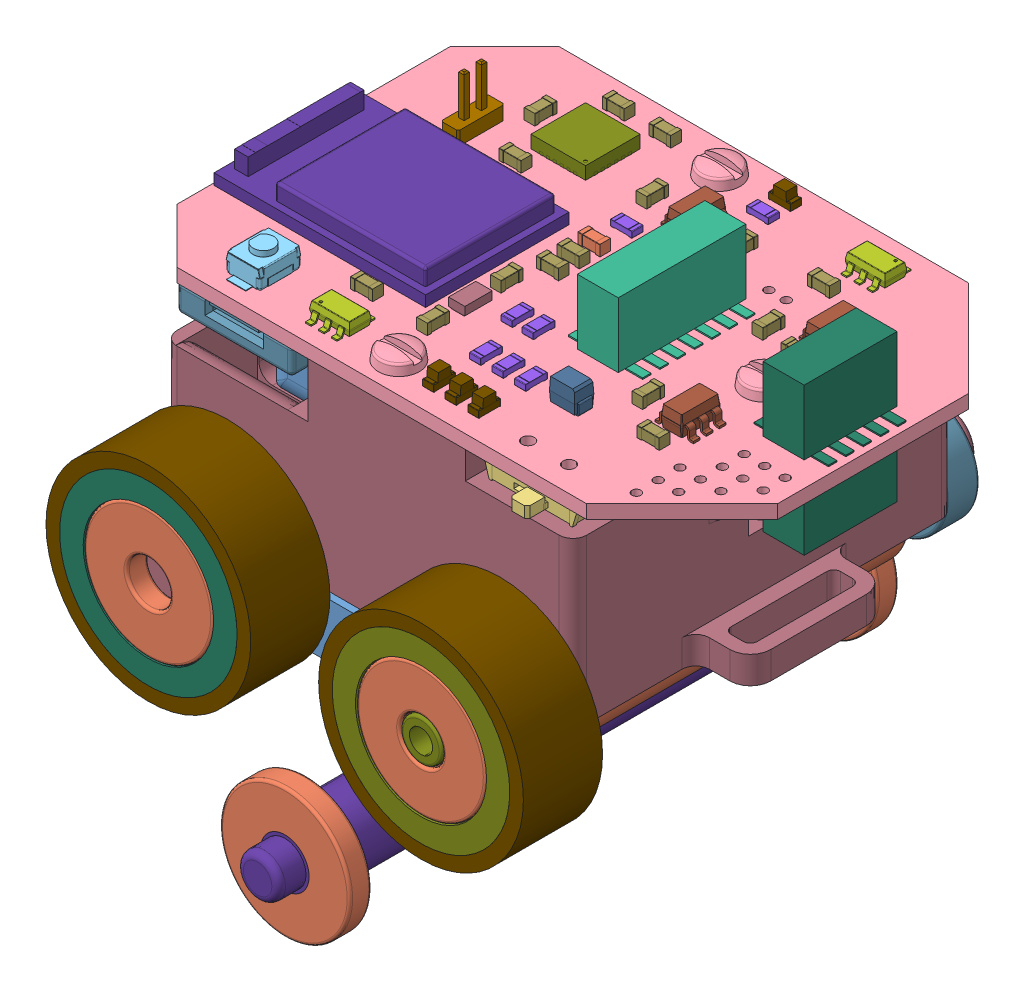
SolidWorks assembly AstroAnt_small_magnet, configuration Default. Lengths in mm.
Overall size (41 37.39 42.61).
158 component instances, 38 part files, 36 mates.
Components (placement in the parent):
- LiPo_360mAh-1: LiPo_360mAh [Default] at (6.8166 4.9998 44.2756) size (25 7 18)
- PA2-50-1: PA2-50 [Default] at (8.0673 -18.301 41.8029) x (0 0 1) z (0.952879 0.303349 0) size (29.1 8 8)
- PA2-50-2: PA2-50 [Default] at (-4.1563 19.5334 49.6029) x (0 0 -1) z (0.755989 -0.654584 0) size (29.1 8 8)
- 92120A150_Brass Heat-Set Inserts for Plastic-1: 92120A150_Brass Heat-Set Inserts for Plastic [92120A150] at (19.9543 12.4998 45.7029) size (2.56 3.33 2.56)
- 92120A150_Brass Heat-Set Inserts for Plastic-2: 92120A150_Brass Heat-Set Inserts for Plastic [92120A150] at (4.9543 12.4998 33.9529) size (2.56 3.33 2.56)
- 92120A150_Brass Heat-Set Inserts for Plastic-3: 92120A150_Brass Heat-Set Inserts for Plastic [92120A150] at (4.9543 12.4998 57.4529) size (2.56 3.33 2.56)
- 91460A005_METRIC CHEESE HEAD SLOTTED MACHINE SCREW-8: 91460A005_METRIC CHEESE HEAD SLOTTED MACHINE SCREW [91460A005] at (4.9543 14.9998 57.4529) x (1 0 0) z (0 1 0) size (3 3 7.1)
- 91460A005_METRIC CHEESE HEAD SLOTTED MACHINE SCREW-9: 91460A005_METRIC CHEESE HEAD SLOTTED MACHINE SCREW [91460A005] at (4.9543 14.9998 33.9529) x (1 0 0) z (0 1 0) size (3 3 7.1)
- 91460A005_METRIC CHEESE HEAD SLOTTED MACHINE SCREW-10: 91460A005_METRIC CHEESE HEAD SLOTTED MACHINE SCREW [91460A005] at (19.9543 14.9998 45.7029) x (1 0 0) z (0 1 0) size (3 3 7.1)
- 92120A150_Brass Heat-Set Inserts for Plastic-4: 92120A150_Brass Heat-Set Inserts for Plastic [92120A150] at (4.9543 1.4998 57.4529) x (-0.616962 0 -0.786993) z (0.786993 0 -0.616962) size (2.56 3.33 2.56)
- 92120A150_Brass Heat-Set Inserts for Plastic-5: 92120A150_Brass Heat-Set Inserts for Plastic [92120A150] at (4.9543 1.4998 33.9529) x (-0.616962 0 -0.786993) z (0.786993 0 -0.616962) size (2.56 3.33 2.56)
- 91460A005_METRIC CHEESE HEAD SLOTTED MACHINE SCREW-14: 91460A005_METRIC CHEESE HEAD SLOTTED MACHINE SCREW [91460A005] at (4.9543 -2.5002 57.4529) x (0.663599 0 0.748089) z (0 -1 0) size (3 3 7.1)
- 91460A005_METRIC CHEESE HEAD SLOTTED MACHINE SCREW-15: 91460A005_METRIC CHEESE HEAD SLOTTED MACHINE SCREW [91460A005] at (4.9543 -2.5002 33.9529) x (0.663599 0 0.748089) z (0 -1 0) size (3 3 7.1)
- mainboard_v1.step-1: mainboard_v1.step [Default] at (-103.0457 13.9998 235.7029) x (0 0 -1) z (0 1 0) size (29.41 41 10.8)
  - B3U-1000P.step-1: B3U-1000P.step [Default] at (178.95 -97.38 1.05) x (1 0 0) z (0 -1 0) size (4 1.75 2.5)
    - COMPOUND.step-1: COMPOUND.step [Default] at origin size (4 1.75 2.5)
  - 20021321-00014C1LF.step-1: 20021321-00014C1LF.step [Default] at (190 -115.5 1.05) size (9.35 5.45 4.85)
    - COMPOUND-0.step-1: COMPOUND-0.step [Default] at origin size (9.35 5.45 4.85)
  - MP6513GJ-Z.step-1: MP6513GJ-Z.step [Default] at (201.21 -120 1.05) x (-1 0 0) z (0 0 1) size (2.8 2.9 1)
    - COMPOUND-1.step-1: COMPOUND-1.step [Default] at origin size (2.8 2.9 1)
  - MP6513GJ-Z.step-2: MP6513GJ-Z.step [Default] at (178.51 -103.46 1.05) size (2.8 2.9 1)
    - COMPOUND-1.step-1: COMPOUND-1.step [Default] at origin size (2.8 2.9 1)
  - R_0603_1608Metric.step-1: R_0603_1608Metric.step [Default] at (195.55 -104.38 -0.05) x (1 0 0) z (0 0 -1) size (1.6 0.8 0.45)
    - SOLID.step-1: SOLID.step [Default] at origin size (1.6 0.8 0.45)
  - R_0603_1608Metric.step-2: R_0603_1608Metric.step [Default] at (192.6 -99.86 -0.05) x (0 1 0) z (0 0 -1) size (1.6 0.8 0.45)
    - SOLID.step-1: SOLID.step [Default] at origin size (1.6 0.8 0.45)
  - PinHeader_2x01_P1.27mm_Vertical.step-1: PinHeader_2x01_P1.27mm_Vertical.step [Default] at (194.96 -96.07 1.05) size (3.4 1.27 6.3)
    - SOLID-2.step-1: SOLID-2.step [Default] at origin size (3.4 1.27 6.3)
  - TAJP106K010RNJ.step-1: TAJP106K010RNJ.step [Default] at (196.22 -98.14 -0.05) x (-1 0 0) z (0 0 -1) size (2.05 1.4 1.7)
    - COMPOUND-3.step-1: COMPOUND-3.step [Default] at origin size (2.05 1.4 1.7)
  - TAJP106K010RNJ.step-2: TAJP106K010RNJ.step [Default] at (181.68 -117.23 1.05) x (0 1 0) z (0 0 1) size (2.05 1.4 1.7)
    - COMPOUND-3.step-1: COMPOUND-3.step [Default] at origin size (2.05 1.4 1.7)
  - SOT-23-5.step-1: SOT-23-5.step [Default] at (195.38 -122.78 1.05) x (0 1 0) z (0 0 1) size (2.8 2.9 1.55)
    - SOLID-4.step-1: SOLID-4.step [Default] at origin size (2.8 2.9 1.55)
  - C_0603_1608Metric.step-1: C_0603_1608Metric.step [Default] at (192.91 -122.55 1.05) x (0 -1 0) z (0 0 1) size (1.6 0.8 0.8)
    - SOLID-5.step-1: SOLID-5.step [Default] at origin size (1.6 0.8 0.8)
  - C_0603_1608Metric.step-2: C_0603_1608Metric.step [Default] at (193.57 -119.76 1.05) size (1.6 0.8 0.8)
    - SOLID-5.step-1: SOLID-5.step [Default] at origin size (1.6 0.8 0.8)
  - ECS-.327-12.5-12-TR.step-1: ECS-.327-12.5-12-TR.step [Default] at (184.31 -107.18 1.05) size (2 1.2 0.7)
    - COMPOUND-6.step-1: COMPOUND-6.step [Default] at origin size (2 1.2 0.7)
  - C_0603_1608Metric.step-3: C_0603_1608Metric.step [Default] at (197.67 -113.69 1.05) size (1.6 0.8 0.8)
    - SOLID-5.step-1: SOLID-5.step [Default] at origin size (1.6 0.8 0.8)
  - C_0603_1608Metric.step-4: C_0603_1608Metric.step [Default] at (197.64 -107.18 1.05) size (1.6 0.8 0.8)
    - SOLID-5.step-1: SOLID-5.step [Default] at origin size (1.6 0.8 0.8)
  - C_0603_1608Metric.step-5: C_0603_1608Metric.step [Default] at (190.96 -108.09 1.05) x (0 1 0) z (0 0 1) size (1.6 0.8 0.8)
    - SOLID-5.step-1: SOLID-5.step [Default] at origin size (1.6 0.8 0.8)
  - 1734592-6.step-1: 1734592-6.step [Default] at (203.79 -118 -1.05) x (0 -1 0) z (1 0 0) size (8.43 2.05 5.11)
    - SOLID-7.step-1: SOLID-7.step [Default] at origin size (8.43 2.05 5.11)
  - 1734592-6.step-2: 1734592-6.step [Default] at (176.19 -98 -1.05) x (0 1 0) z (-1 0 0) size (8.43 2.05 5.11)
    - SOLID-7.step-1: SOLID-7.step [Default] at origin size (8.43 2.05 5.11)
  - 20021321-00010C4LF.step-1: 20021321-00010C4LF.step [Default] at (190 -127.85 -0.05) x (1 0 0) z (0 0 -1) size (6.81 5.45 4.85)
    - COMPOUND-8.step-1: COMPOUND-8.step [Default] at origin size (6.81 5.45 4.85)
  - 20021321-00010C4LF.step-2: 20021321-00010C4LF.step [Default] at (190 -127.85 1.05) size (6.81 5.45 4.85)
    - COMPOUND-8.step-1: COMPOUND-8.step [Default] at origin size (6.81 5.45 4.85)
  - C_0603_1608Metric.step-6: C_0603_1608Metric.step [Default] at (181.31 -102.6 1.05) x (0 -1 0) z (0 0 1) size (1.6 0.8 0.8)
    - SOLID-5.step-1: SOLID-5.step [Default] at origin size (1.6 0.8 0.8)
  - C_0603_1608Metric.step-7: C_0603_1608Metric.step [Default] at (198.25 -119.14 1.05) x (0 -1 0) z (0 0 1) size (1.6 0.8 0.8)
    - SOLID-5.step-1: SOLID-5.step [Default] at origin size (1.6 0.8 0.8)
  - MPU6050.step-1: MPU6050.step [Default] at (198.43 -101.5 1.05) x (0 1 0) z (1 0 0) size (4 0.95 4)
    - COMPOUND-9.step-1: COMPOUND-9.step [Default] at origin size (4 0.95 4)
  - C_0603_1608Metric.step-8: C_0603_1608Metric.step [Default] at (194.9 -99.89 1.05) x (0 -1 0) z (0 0 1) size (1.6 0.8 0.8)
    - SOLID-5.step-1: SOLID-5.step [Default] at origin size (1.6 0.8 0.8)
  - C_0603_1608Metric.step-9: C_0603_1608Metric.step [Default] at (201.98 -100.38 1.05) x (0 -1 0) z (0 0 1) size (1.6 0.8 0.8)
    - SOLID-5.step-1: SOLID-5.step [Default] at origin size (1.6 0.8 0.8)
  - C_0603_1608Metric.step-10: C_0603_1608Metric.step [Default] at (201.98 -103.78 1.05) x (0 1 0) z (0 0 1) size (1.6 0.8 0.8)
    - SOLID-5.step-1: SOLID-5.step [Default] at origin size (1.6 0.8 0.8)
  - C_0603_1608Metric.step-11: C_0603_1608Metric.step [Default] at (198.81 -97.82 1.05) size (1.6 0.8 0.8)
    - SOLID-5.step-1: SOLID-5.step [Default] at origin size (1.6 0.8 0.8)
  - SOT-23-5.step-2: SOT-23-5.step [Default] at (184.86 -122.77 1.05) x (0 1 0) z (0 0 1) size (2.8 2.9 1.55)
    - SOLID-4.step-1: SOLID-4.step [Default] at origin size (2.8 2.9 1.55)
  - SOT-23-5.step-3: SOT-23-5.step [Default] at (197.58 -110.46 1.05) x (0 1 0) z (0 0 1) size (2.8 2.9 1.55)
    - SOLID-4.step-1: SOLID-4.step [Default] at origin size (2.8 2.9 1.55)
  - MDBT50Q-1MV2.step-1: MDBT50Q-1MV2.step [Default] at (187.3136 -98.605 1.0754) x (-1 0 0) z (0 1 0) size (10.5 2.06 15.5)
    - SOLID-10.step-1: SOLID-10.step [Default] at origin size (10.5 2.06 15.5)
  - C_0603_1608Metric.step-12: C_0603_1608Metric.step [Default] at (189.44 -108.09 1.05) x (0 1 0) z (0 0 1) size (1.6 0.8 0.8)
    - SOLID-5.step-1: SOLID-5.step [Default] at origin size (1.6 0.8 0.8)
  - C_0603_1608Metric.step-13: C_0603_1608Metric.step [Default] at (181.57 -107.18 1.05) x (-1 0 0) z (0 0 1) size (1.6 0.8 0.8)
    - SOLID-5.step-1: SOLID-5.step [Default] at origin size (1.6 0.8 0.8)
  - C_0603_1608Metric.step-14: C_0603_1608Metric.step [Default] at (186.97 -107.18 1.05) size (1.6 0.8 0.8)
    - SOLID-5.step-1: SOLID-5.step [Default] at origin size (1.6 0.8 0.8)
  - C_0603_1608Metric.step-15: C_0603_1608Metric.step [Default] at (184.77 -119.75 1.05) x (-1 0 0) z (0 0 1) size (1.6 0.8 0.8)
    - SOLID-5.step-1: SOLID-5.step [Default] at origin size (1.6 0.8 0.8)
  - C_0603_1608Metric.step-16: C_0603_1608Metric.step [Default] at (182.37 -122.54 1.05) x (0 -1 0) z (0 0 1) size (1.6 0.8 0.8)
    - SOLID-5.step-1: SOLID-5.step [Default] at origin size (1.6 0.8 0.8)
  - LED_0603_1608Metric.step-1: LED_0603_1608Metric.step [Default] at (178.19 -111.01 1.05) size (1.6 0.8 1.1)
    - SOLID-11.step-1: SOLID-11.step [Default] at origin size (1.6 0.8 1.1)
  - LED_0603_1608Metric.step-2: LED_0603_1608Metric.step [Default] at (178.19 -112.66 1.05) size (1.6 0.8 1.1)
    - SOLID-11.step-1: SOLID-11.step [Default] at origin size (1.6 0.8 1.1)
  - LED_0603_1608Metric.step-3: LED_0603_1608Metric.step [Default] at (178.19 -114.31 1.05) size (1.6 0.8 1.1)
    - SOLID-11.step-1: SOLID-11.step [Default] at origin size (1.6 0.8 1.1)
  - LED_0603_1608Metric.step-4: LED_0603_1608Metric.step [Default] at (202.34 -112.21 1.05) x (0 1 0) z (0 0 1) size (1.6 0.8 1.1)
    - SOLID-11.step-1: SOLID-11.step [Default] at origin size (1.6 0.8 1.1)
  - 473460001.step-1: 473460001.step [Default] at (201.68 -99.72 -1.25) x (0 -1 0) z (1 0 0) size (7.98 2.94 5.43)
    - COMPOUND-12.step-1: COMPOUND-12.step [Default] at origin size (7.98 2.94 5.43)
  - L_0603_1608Metric.step-1: L_0603_1608Metric.step [Default] at (192.48 -108.09 1.05) x (0 1 0) z (0 0 1) size (1.6 0.8 0.8)
    - SOLID-13.step-1: SOLID-13.step [Default] at origin size (1.6 0.8 0.8)
  - R_0603_1608Metric.step-3: R_0603_1608Metric.step [Default] at (185.18 -111.31 1.05) x (-1 0 0) z (0 0 1) size (1.6 0.8 0.45)
    - SOLID.step-1: SOLID.step [Default] at origin size (1.6 0.8 0.45)
  - R_0603_1608Metric.step-4: R_0603_1608Metric.step [Default] at (185.18 -109.77 1.05) size (1.6 0.8 0.45)
    - SOLID.step-1: SOLID.step [Default] at origin size (1.6 0.8 0.45)
  - R_0603_1608Metric.step-5: R_0603_1608Metric.step [Default] at (181.62 -111.01 1.05) size (1.6 0.8 0.45)
    - SOLID.step-1: SOLID.step [Default] at origin size (1.6 0.8 0.45)
  - R_0603_1608Metric.step-6: R_0603_1608Metric.step [Default] at (181.62 -112.66 1.05) size (1.6 0.8 0.45)
    - SOLID.step-1: SOLID.step [Default] at origin size (1.6 0.8 0.45)
  - R_0603_1608Metric.step-7: R_0603_1608Metric.step [Default] at (181.62 -114.31 1.05) x (-1 0 0) z (0 0 1) size (1.6 0.8 0.45)
    - SOLID.step-1: SOLID.step [Default] at origin size (1.6 0.8 0.45)
  - R_0603_1608Metric.step-8: R_0603_1608Metric.step [Default] at (194.84 -108.1 1.05) x (0 1 0) z (0 0 1) size (1.6 0.8 0.45)
    - SOLID.step-1: SOLID.step [Default] at origin size (1.6 0.8 0.45)
  - R_0603_1608Metric.step-9: R_0603_1608Metric.step [Default] at (200.69 -112.2325 1.05) x (0 1 0) z (0 0 1) size (1.6 0.8 0.45)
    - SOLID.step-1: SOLID.step [Default] at origin size (1.6 0.8 0.45)
  - R_0603_1608Metric.step-10: R_0603_1608Metric.step [Default] at (196.22 -101.51 -0.05) x (-1 0 0) z (0 0 -1) size (1.6 0.8 0.45)
    - SOLID.step-1: SOLID.step [Default] at origin size (1.6 0.8 0.45)
  - R_0603_1608Metric.step-11: R_0603_1608Metric.step [Default] at (196.22 -99.9725 -0.05) x (-1 0 0) z (0 0 -1) size (1.6 0.8 0.45)
    - SOLID.step-1: SOLID.step [Default] at origin size (1.6 0.8 0.45)
  - SW_SPDT_PCM12.step-1: SW_SPDT_PCM12.step [Default] at (178.18 -119.37 -0.05) x (0 1 0) z (0 0 -1) size (7.7 5 2)
    - SOLID-14.step-1: SOLID-14.step [Default] at origin size (7.7 5 2)
  - COMPOUND-15.step-1: COMPOUND-15.step [Default] at origin size (28 41 1)
- 91613A020_METRIC CHEESE HEAD SLOTTED MACHINE SCREW-1: 91613A020_METRIC CHEESE HEAD SLOTTED MACHINE SCREW [91613A020] at (1.2533 -0.5002 54.4029) x (1 0 0) z (0 1 0) size (3 3 5.08)
- 91613A020_METRIC CHEESE HEAD SLOTTED MACHINE SCREW-2: 91613A020_METRIC CHEESE HEAD SLOTTED MACHINE SCREW [91613A020] at (8.6533 -0.5002 54.4029) x (1 0 0) z (0 1 0) size (3 3 5.08)
- 91613A020_METRIC CHEESE HEAD SLOTTED MACHINE SCREW-3: 91613A020_METRIC CHEESE HEAD SLOTTED MACHINE SCREW [91613A020] at (1.2533 -0.5002 37.0029) x (1 0 0) z (0 1 0) size (3 3 5.08)
- IR_TEMP_V2.step-3: IR_TEMP_V2.step [Default] at (118.9553 -0.5002 109.7029) x (-1 0 0) z (0 1 0) size (10 20 4.8)
  - Board_Geoms_380f.step-1: Board_Geoms_380f.step [Default] at origin size (10 20 1.11)
    - Pcb_380f.step-1: Pcb_380f.step [Default] at origin size (10 20 1)
    - topTracks_380f.step-1: topTracks_380f.step [Default] at (0 0 0.01) size (9.62 17.53 0.05)
    - botTracks_380f.step-1: botTracks_380f.step [Default] at (0 0 -1.01) size (9.25 16.88 0.05)
  - Step_Models_380f.step-1: Step_Models_380f.step [Default] at origin size (9.46 10.17 4.8)
    - Top_380f.step-1: Top_380f.step [Default] at origin size (9.46 10.17 1.2)
      - IC1_PW14_613E6C6D.step-1: IC1_PW14_613E6C6D.step [Default] at (113.99 -59.48 0) x (-1 0 0) z (0 1 0) size (6.4 1.2 5)
      - C1_C_0402_1005Metric_613EDDF6.step-1: C1_C_0402_1005Metric_613EDDF6.step [Default] at (110.5 -64.26 0) x (-1 0 0) z (0 0 1) size (1 0.5 0.5)
      - C1_C_0402_1005Metric_613EDDF6.step-2: C1_C_0402_1005Metric_613EDDF6.step [Default] at (109.52 -61.07 0) x (0 -1 0) z (0 0 1) size (1 0.5 0.5)
      - C1_C_0402_1005Metric_613EDDF6.step-3: C1_C_0402_1005Metric_613EDDF6.step [Default] at (118.48 -60.86 0) x (0 -1 0) z (0 0 1) size (1 0.5 0.5)
      - C1_C_0402_1005Metric_613EDDF6.step-4: C1_C_0402_1005Metric_613EDDF6.step [Default] at (118.48 -58.59 0) x (0 -1 0) z (0 0 1) size (1 0.5 0.5)
      - C1_C_0402_1005Metric_613EDDF6.step-5: C1_C_0402_1005Metric_613EDDF6.step [Default] at (113.32 -66.9 0) size (1 0.5 0.5)
      - R1_R_0402_1005Metric_613EDE7A.step-1: R1_R_0402_1005Metric_613EDE7A.step [Default] at (110.98 -63.1 0) size (1 0.5 0.35)
      - R1_R_0402_1005Metric_613EDE7A.step-2: R1_R_0402_1005Metric_613EDE7A.step [Default] at (111.68 -66.3 0) x (0 1 0) z (0 0 1) size (1 0.5 0.35)
    - Bot_380f.step-1: Bot_380f.step [Default] at origin size (6.35 7.64 4.6)
      - U1_ZTP-135SR_613E6CD4.step-1: U1_ZTP-135SR_613E6CD4.step [Default] at (114 -64 -1) x (-1 0 0) z (0 -1 0) size (6.35 4.6 5.4)
      - C1_C_0402_1005Metric_613EDDF6.step-1: C1_C_0402_1005Metric_613EDDF6.step [Default] at (115.07 -59.56 -1) x (0 -1 0) z (0 0 -1) size (1 0.5 0.5)
      - R1_R_0402_1005Metric_613EDE7A.step-1: R1_R_0402_1005Metric_613EDE7A.step [Default] at (113.64 -59.58 -1) x (0 -1 0) z (0 0 -1) size (1 0.5 0.35)
- Body_simple-1: Body_simple [Default] at (4.8007 -0.0002 38.7677) size (34 16 37)
- ball_bearing_5x11x4mm-1: ball_bearing_5x11x4mm [Default] at (-45.4624 -2.1758 28.9029) x (0.999925 -0.012245 0) z (0 0 1) size (8 8 2.5)
- wheel_holder_non_motor-1: wheel_holder_non_motor [Default] at (-70.2522 1.7638 25.6029) size (13 13 5.8) (hidden)
- wheel_holder_non_motor-2: wheel_holder_non_motor [Default] at (-19.1131 -84.0559 65.8029) x (0.185441 0.982655 0) z (0 0 -1) size (13 13 5.8)
- ball_bearing_5x11x4mm-2: ball_bearing_5x11x4mm [Default] at (-30.2803 -54.9376 62.5029) x (0.373101 0.927791 0) z (0 0 -1) size (8 8 2.5)
- wheel_motor-1: wheel_motor [Default] at (24.0366 1.7037 25.5779) size (13 13 5.8) (hidden)
- wheel_motor-2: wheel_motor [Default] at (15.5431 29.126 65.8279) x (-0.038296 0.999266 0) z (0 0 -1) size (13 13 5.8)
- magnet_wheel_holder-1: magnet_wheel_holder [Default] at (28.927 0.8494 27.1904) size (5 5 42.61)
- tire-1: tire [Default] at (38.167 -1.442 25.5779) size (15 15 5.8) (hidden)
- tire-2: tire [Default] at (58.167 -1.442 25.6029) size (15 15 5.8) (hidden)
- tire-3: tire [Default] at (38.167 -1.442 60.0029) size (15 15 5.8)
- tire-4: tire [Default] at (58.167 -1.442 60.0279) size (15 15 5.8)
- motor_holder-2: motor_holder [Default] at (-0.192 -4.5002 11.9282) size (20 4.13 28)
- R8201-1: R8201 [Default] at (-53.4439 -3.2146 25.6029) size (9.53 9.53 1.59) (hidden)
- R8201-2: R8201 [Default] at (-73.4439 -3.2146 25.5779) size (9.53 9.53 1.59) (hidden)
- R8201-3: R8201 [Default] at (-53.4439 -3.2146 64.2404) size (9.53 9.53 1.59)
- R8201-4: R8201 [Default] at (-73.4439 -3.2146 64.2154) size (9.53 9.53 1.59)
- R8201-5: R8201 [Default] at (-63.4439 -15.9439 25.6029) size (9.53 9.53 1.59)
- R8201-6: R8201 [Default] at (-63.4439 -15.9439 64.2154) size (9.53 9.53 1.59)
Mates (geometry in assembly coordinates):
- Coincident100: coincident anti-aligned: plane of mainboard_v1.step-1/COMPOUND-15.step-1 through (6.7692 13.9998 45.7029) normal (0 -1 0); plane of Body_simple-1 through (4.8007 13.9998 38.7677) normal (0 1 0)
- Concentric58: concentric anti-aligned: cylinder of PA2-50-2 through (-5.0457 -0.0002 33.4029) axis (0 0 1) radius 4; cylinder of Body_simple-1 through (-5.0457 -0.0002 57.7029) axis (0 0 -1) radius 4.1
- Concentric59: concentric aligned: cylinder of mainboard_v1.step-1/COMPOUND-15.step-1 through (19.9543 13.4998 45.7029) axis (0 1 0) radius 0.85; cylinder of Body_simple-1 through (19.9543 5.9998 45.7029) axis (0 1 0) radius 1.15
- Concentric63: concentric anti-aligned: cylinder of ball_bearing_5x11x4mm-1 through (14.9543 -0.0002 31.4029) axis (0 0 -1) radius 4; cylinder of wheel_holder_non_motor-1 through (14.9543 -0.0002 25.6029) axis (0 0 1) radius 4
- Concentric66: concentric anti-aligned: cylinder of Body_simple-1 through (14.9543 -0.0002 27.2029) axis (0 0 1) radius 2; cylinder of ball_bearing_5x11x4mm-1 through (14.9543 -0.0002 32.9029) axis (0 0 -1) radius 2
- Distance2: distance = 0.3 mm anti-aligned: plane of wheel_holder_non_motor-1 through (14.9543 -0.0002 31.4029) normal (0 0 1); plane of Body_simple-1 through (-10.0457 13.9998 31.7029) normal (0 0 -1)
- Coincident105: coincident aligned: plane of ball_bearing_5x11x4mm-1 through (14.9543 -0.0002 31.4029) normal (0 0 1); plane of wheel_holder_non_motor-1 through (14.9543 -0.0002 31.4029) normal (0 0 1)
- Distance3: distance = 0.3 mm anti-aligned: plane of wheel_holder_non_motor-2 through (-5.0457 -0.0002 60.0029) normal (0 0 -1); plane of Body_simple-1 through (-10.0457 13.9998 59.7029) normal (0 0 1)
- Concentric67: concentric aligned: cylinder of Body_simple-1 through (-5.0457 -0.0002 64.2029) axis (0 0 -1) radius 2; cylinder of wheel_holder_non_motor-2 through (-5.0457 -0.0002 65.8029) axis (0 0 -1) radius 4
- Coincident107: coincident aligned: plane of wheel_holder_non_motor-2 through (-5.0457 -0.0002 60.0029) normal (0 0 -1); plane of ball_bearing_5x11x4mm-2 through (-5.0457 -0.0002 60.0029) normal (0 0 -1)
- Concentric68: concentric anti-aligned: cylinder of Body_simple-1 through (-5.0457 -0.0002 64.2029) axis (0 0 -1) radius 2; cylinder of ball_bearing_5x11x4mm-2 through (-5.0457 -0.0002 58.5029) axis (0 0 1) radius 2
- Concentric83: concentric anti-aligned: cylinder of wheel_motor-1 through (-5.0457 -0.0002 31.3779) axis (0 0 -1) radius 6.5; cylinder of tire-1 through (-5.0457 -0.0002 25.5779) axis (0 0 1) radius 6.5
- Coincident123: coincident aligned: plane of wheel_motor-1 through (-5.0457 -0.0002 25.5779) normal (0 0 -1); plane of tire-1 through (-5.0457 -0.0002 25.5779) normal (0 0 -1)
- Concentric84: concentric anti-aligned: cylinder of wheel_holder_non_motor-1 through (14.9543 -0.0002 31.4029) axis (0 0 -1) radius 6.5; cylinder of tire-2 through (14.9543 -0.0002 25.6029) axis (0 0 1) radius 6.5
- Coincident124: coincident aligned: plane of wheel_holder_non_motor-1 through (14.9543 -0.0002 25.6029) normal (0 0 -1); plane of tire-2 through (14.9543 -0.0002 25.6029) normal (0 0 -1)
- Coincident125: coincident aligned: plane of wheel_motor-2 through (14.9543 -0.0002 65.8279) normal (0 0 1); plane of tire-4 through (14.9543 -0.0002 65.8279) normal (0 0 1)
- Concentric85: concentric aligned: cylinder of wheel_motor-2 through (14.9543 -0.0002 60.0279) axis (0 0 1) radius 6.5; cylinder of tire-4 through (14.9543 -0.0002 60.0279) axis (0 0 1) radius 6.5
- Coincident126: coincident aligned: plane of wheel_holder_non_motor-2 through (-5.0457 -0.0002 65.8029) normal (0 0 1); plane of tire-3 through (-5.0457 -0.0002 65.8029) normal (0 0 1)
- Concentric86: concentric aligned: cylinder of wheel_holder_non_motor-2 through (-5.0457 -0.0002 60.0029) axis (0 0 1) radius 6.5; cylinder of tire-3 through (-5.0457 -0.0002 60.0029) axis (0 0 1) radius 6.5
- Concentric94: concentric anti-aligned: cylinder of IR_TEMP_V2.step-3/Step_Models_380f.step-1/Bot_380f.step-1/U1_ZTP-135SR_613E6CD4.step-1 through (4.9553 -4.1002 45.7029) axis (0 1 0) radius 2.35; cylinder of motor_holder-2 through (4.9553 -0.5002 45.7029) axis (0 -1 0) radius 2.5
- Coincident128: coincident anti-aligned: plane of IR_TEMP_V2.step-3/Board_Geoms_380f.step-1/Pcb_380f.step-1 through (4.9553 -1.5002 45.7029) normal (0 -1 0); plane of motor_holder-2 through (-0.192 -1.5002 11.9282) normal (0 1 0)
- Concentric95: concentric anti-aligned: cylinder of Body_simple-1 through (14.9543 -0.0002 27.2029) axis (0 0 1) radius 2; cylinder of R8201-1 through (14.9543 -0.0002 27.1904) axis (0 0 -1) radius 1.5875
- Concentric96: concentric aligned: cylinder of wheel_motor-1 through (-5.0457 -0.0002 28.5779) axis (0 0 -1) radius 1.525; cylinder of R8201-2 through (-5.0457 -0.0002 27.1654) axis (0 0 -1) radius 1.5875
- Concentric97: concentric anti-aligned: cylinder of wheel_motor-2 through (14.9543 -0.0002 62.8279) axis (0 0 1) radius 1.525; cylinder of R8201-3 through (14.9543 -0.0002 65.8279) axis (0 0 -1) radius 1.5875
- Concentric98: concentric aligned: cylinder of Body_simple-1 through (-5.0457 -0.0002 64.2029) axis (0 0 -1) radius 2; cylinder of R8201-4 through (-5.0457 -0.0002 65.8029) axis (0 0 -1) radius 1.5875
- Coincident130: coincident aligned: plane of wheel_holder_non_motor-2 through (-5.0457 -0.0002 65.8029) normal (0 0 1); plane of R8201-4 through (-5.0457 -0.0002 65.8029) normal (0 0 1)
- Coincident131: coincident aligned: plane of wheel_motor-1 through (-5.0457 -0.0002 25.5779) normal (0 0 -1); plane of R8201-2 through (-5.0457 -0.0002 25.5779) normal (0 0 -1)
- Coincident132: coincident aligned: plane of wheel_holder_non_motor-1 through (14.9543 -0.0002 25.6029) normal (0 0 -1); plane of R8201-1 through (14.9543 -0.0002 25.6029) normal (0 0 -1)
- Concentric99: concentric anti-aligned: cylinder of PA2-50-1 through (14.9543 -0.0002 63.1029) axis (0 0 -1) radius 0.5; cylinder of wheel_motor-2 through (14.9543 -0.0002 60.0279) axis (0 0 1) radius 0.85
- Concentric100: concentric anti-aligned: cylinder of PA2-50-2 through (-5.0457 -0.0002 28.3029) axis (0 0 1) radius 0.5; cylinder of wheel_motor-1 through (-5.0457 -0.0002 31.3779) axis (0 0 -1) radius 0.85
- Concentric101: concentric aligned: cylinder of magnet_wheel_holder-1 through (4.9543 -12.7295 67.8004) axis (0 0 -1) radius 1.55; cylinder of R8201-6 through (4.9543 -12.7295 65.8029) axis (0 0 -1) radius 1.5875
- Concentric102: concentric anti-aligned: cylinder of magnet_wheel_holder-1 through (4.9543 -12.7295 25.1904) axis (0 0 1) radius 1.55; cylinder of R8201-5 through (4.9543 -12.7295 27.1904) axis (0 0 -1) radius 1.5875
- Coincident133: coincident aligned: plane of wheel_holder_non_motor-1 through (14.9543 -0.0002 25.6029) normal (0 0 -1); plane of R8201-5 through (4.9543 -12.7295 25.6029) normal (0 0 -1)
- Coincident134: coincident aligned: plane of wheel_holder_non_motor-2 through (-5.0457 -0.0002 65.8029) normal (0 0 1); plane of R8201-6 through (4.9543 -12.7295 65.8029) normal (0 0 1)
- Coincident135: coincident aligned: plane of wheel_motor-2 through (14.9543 -0.0002 65.8279) normal (0 0 1); plane of R8201-3 through (14.9543 -0.0002 65.8279) normal (0 0 1)
- Coincident139: coincident anti-aligned: plane of magnet_wheel_holder-1 through (4.9543 -12.7295 27.1904) normal (0 0 -1); plane of R8201-5 through (4.9543 -12.7295 27.1904) normal (0 0 1)
